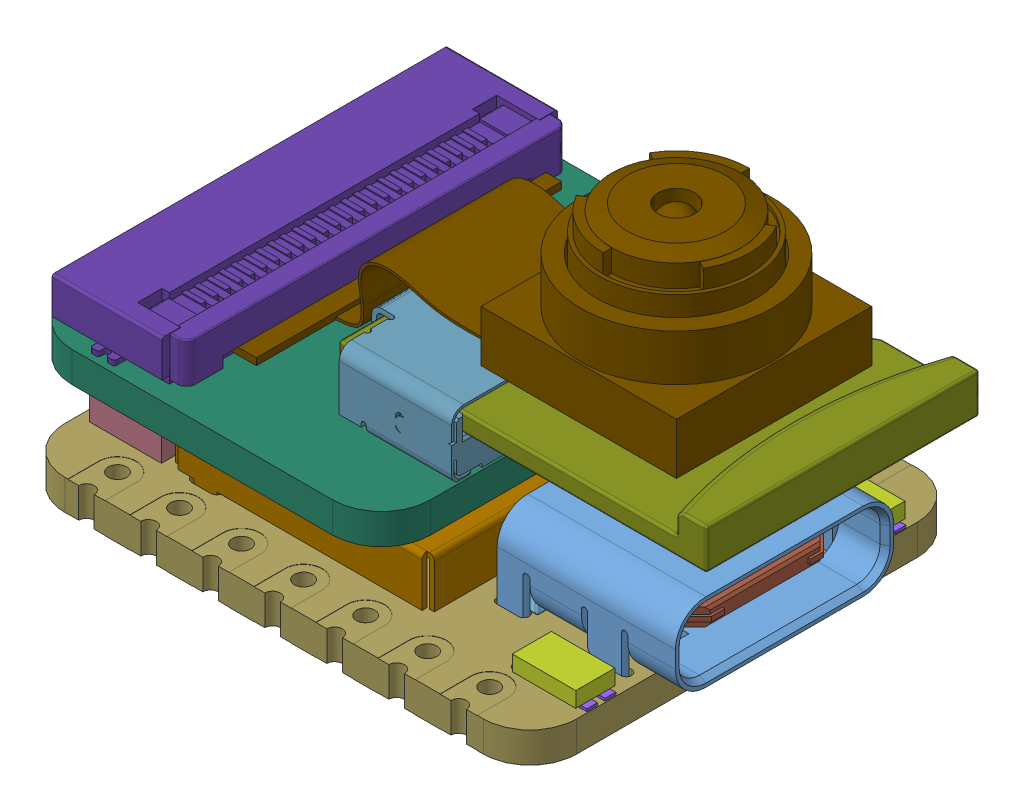
SolidWorks assembly Seeed Studio XIAO-ESP32-S3-Sense, configuration Default. Lengths in mm.
Overall size (24.36 13.98 17.79).
45 component instances, 36 part files, 0 mates.
Components (placement in the parent):
- Seeed Studio XIAO-ESP32-S3-Sense.step-1: Seeed Studio XIAO-ESP32-S3-Sense.step [Default] at origin size (24.36 13.98 17.79)
  - Seeed Studio XIAO-ESP32-S3 (Sense).step-1: Seeed Studio XIAO-ESP32-S3 (Sense).step [Default] at origin size (22.49 4.48 17.79)
    - USB TYPE C PORT.step-1: USB TYPE C PORT.step [Default] at (4.3161 13.395 -12.1571) x (0 0 -1) z (0 -1 0) size (8.94 7.9 4.2)
      - USB TYPE C PORT (1).step-1: USB TYPE C PORT (1).step [Default] at (-3.0192 1.0963 5.395) size (8.94 7.9 4.2)
        - BOSS-EXTRUDE14_8_.step-1: BOSS-EXTRUDE14_8_.step [Default] at (-3.0192 1.0963 5.395) size (0.6 1 0.3)
        - BOSS-EXTRUDE7_4_.step-1: BOSS-EXTRUDE7_4_.step [Default] at (-3.0192 1.0963 5.395) size (0.3 3.78 0.75)
        - BOSS-EXTRUDE7_3_.step-1: BOSS-EXTRUDE7_3_.step [Default] at (-3.0192 1.0963 5.395) size (0.3 3.78 0.75)
        - BOSS-EXTRUDE14_4_.step-1: BOSS-EXTRUDE14_4_.step [Default] at (-3.0192 1.0963 5.395) size (0.3 1 0.3)
        - BOSS-EXTRUDE14_2_.step-1: BOSS-EXTRUDE14_2_.step [Default] at (-3.0192 1.0963 5.395) size (0.6 1 0.3)
        - BOSS-EXTRUDE14_11_.step-1: BOSS-EXTRUDE14_11_.step [Default] at (-3.0192 1.0963 5.395) size (0.3 1 0.3)
        - BOSS-EXTRUDE7_7_.step-1: BOSS-EXTRUDE7_7_.step [Default] at (-3.0192 1.0963 5.395) size (0.3 3.78 0.75)
        - BOSS-EXTRUDE14_9_.step-1: BOSS-EXTRUDE14_9_.step [Default] at (-3.0192 1.0963 5.395) size (0.3 1 0.3)
        - BOSS-EXTRUDE14_3_.step-1: BOSS-EXTRUDE14_3_.step [Default] at (-3.0192 1.0963 5.395) size (0.3 1 0.3)
        - BOSS-EXTRUDE14_7_.step-1: BOSS-EXTRUDE14_7_.step [Default] at (-3.0192 1.0963 5.395) size (0.6 1 0.3)
        - MIRROR2.step-1: MIRROR2.step [Default] at (-3.0192 1.0963 5.395) size (6.7 4.6 0.7)
        - BOSS-EXTRUDE14_5_.step-1: BOSS-EXTRUDE14_5_.step [Default] at (-3.0192 1.0963 5.395) size (0.3 1 0.3)
        - BOSS-EXTRUDE14_12_.step-1: BOSS-EXTRUDE14_12_.step [Default] at (-3.0192 1.0963 5.395) size (0.3 1 0.3)
        - BOSS-EXTRUDE7_8_.step-1: BOSS-EXTRUDE7_8_.step [Default] at (-3.0192 1.0963 5.395) size (0.3 3.78 0.75)
        - BOSS-EXTRUDE7_1_.step-1: BOSS-EXTRUDE7_1_.step [Default] at (-3.0192 1.0963 5.395) size (0.3 3.78 0.75)
        - BOSS-EXTRUDE14_10_.step-1: BOSS-EXTRUDE14_10_.step [Default] at (-3.0192 1.0963 5.395) size (0.3 1 0.3)
        - BOSS-EXTRUDE7_9_.step-1: BOSS-EXTRUDE7_9_.step [Default] at (-3.0192 1.0963 5.395) size (0.3 3.78 0.75)
        - BOSS-EXTRUDE14_6_.step-1: BOSS-EXTRUDE14_6_.step [Default] at (-3.0192 1.0963 5.395) size (0.6 1 0.3)
        - CHAMFER9.step-1: CHAMFER9.step [Default] at (-3.0192 1.0963 5.395) size (8.94 7.3 4.2)
        - BOSS-EXTRUDE14_1_.step-1: BOSS-EXTRUDE14_1_.step [Default] at (-3.0192 1.0963 5.395) size (0.3 1 0.3)
        - BOSS-EXTRUDE7_6_.step-1: BOSS-EXTRUDE7_6_.step [Default] at (-3.0192 1.0963 5.395) size (0.3 3.78 0.75)
        - BOSS-EXTRUDE7_2_.step-1: BOSS-EXTRUDE7_2_.step [Default] at (-3.0192 1.0963 5.395) size (0.3 3.78 0.75)
        - CUT-EXTRUDE5.step-1: CUT-EXTRUDE5.step [Default] at (-3.0192 1.0963 5.395) size (8.54 2 3.59)
        - BOSS-EXTRUDE7_5_.step-1: BOSS-EXTRUDE7_5_.step [Default] at (-3.0192 1.0963 5.395) size (0.3 3.78 0.75)
    - SKTAAAE010 v1.step-1: SKTAAAE010 v1.step [Default] at (10.7092 1 -12.0449) x (1 0 0) z (0 1 0) size (3.09 1.6 0.73)
      - Body.step-1: Body.step [Default] at (0 0 0.1) size (2.6 1.6 0.63)
      - Pins.step-1: Pins.step [Default] at origin size (3.09 1.19 0.1)
    - SKTAAAE010 v1.step-2: SKTAAAE010 v1.step [Default] at (10.6911 1 -0.1868) x (1 0 0) z (0 1 0) size (3.09 1.6 0.73)
      - Body.step-1: Body.step [Default] at (0 0 0.1) size (2.6 1.6 0.63)
      - Pins.step-1: Pins.step [Default] at origin size (3.09 1.19 0.1)
    - Shield.step-1: Shield.step [Default] at origin size (10.6 2.7 12.6)
    - U.FL-R-SMT-1_10_ v1.step-1: U.FL-R-SMT-1_10_ v1.step [Default] at (-6.9517 1 -10.8381) x (1 0 0) z (0 1 0) size (3 3.1 1.25)
    - DF40C-30DP-0.4V_51_ v1.step-1: DF40C-30DP-0.4V_51_ v1.step [Default] at (-6.0667 1.65 -7.7227) size (2.97 1.14 7.52)
    - Seeed Studio XIAO-ESP32-S3 (Sense)-0.step-1: Seeed Studio XIAO-ESP32-S3 (Sense)-0.step [Default] at origin size (20.97 1.28 17.79)
  - Sense Expansion Board.step-1: Sense Expansion Board.step [Default] at (-0.3 4.5 0) x (-1 0 0) z (0 0 1) size (24.36 7.23 16.78)
    - DF40HC(3.0)-30DS.step-1: DF40HC(3.0)-30DS.step [Default] at (6.4217 1.57 -3.0777) x (-1 0 0) z (0 0 1) size (3.38 2.9 8.6)
    - 10067099-200LF v1.step-1: 10067099-200LF v1.step [Default] at (-1.3077 -2.08 -6.0846) x (0 0 -1) z (-1 0 0) size (11.4 2.65 5.5)
    - PCB.step-1: PCB.step [Default] at origin size (14.68 1.25 16.78)
    - MicroSD v2.step-1: MicroSD v2.step [Default] at (-8.16 -2.1 -6.9267) x (1 0 0) z (0 0 -1) size (15.06 1.66 11.19)
    - JUSHUO AFC01-S24FCA-00.step-1: JUSHUO AFC01-S24FCA-00.step [Default] at (6.9932 -0.67 -6.0797) x (0 0 1) z (0 -1 0) size (16.2 6.01 2.01)
  - Camer Module.step-1: Camer Module.step [Default] at (-7.2 6 -13) size (19.95 8.11 12.5)
